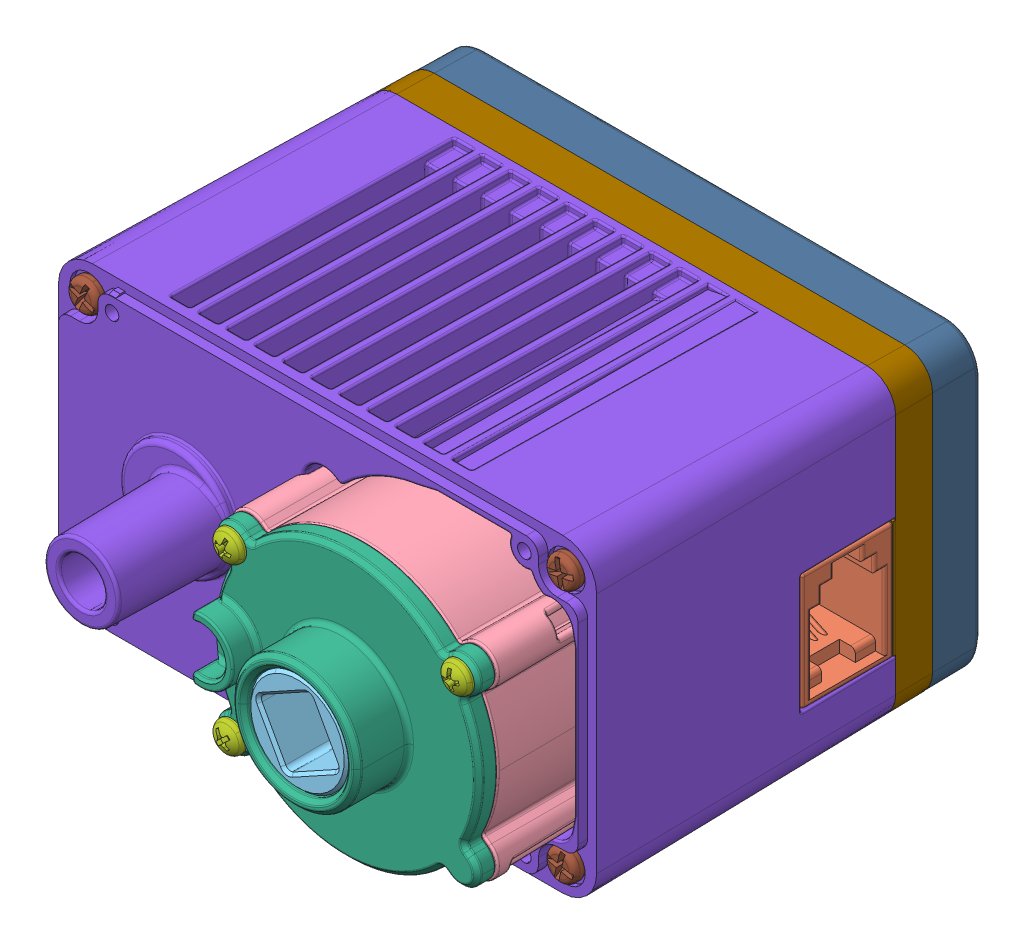
SolidWorks assembly V5 Smart Motor (276-4840) no cap 2, configuration Default. Lengths in mm.
Overall size (59.01 35.33 59.91).
19 component instances, 12 part files, 0 mates.
Components (placement in the parent):
- 276-4840-900 Rev6_Instruction.step-1: 276-4840-900 Rev6_Instruction.step [Default] at (-14.3 0 -17.2) size (52.79 15.94 38.15)
  - 276-4840-901 Rev6.step-1: 276-4840-901 Rev6.step [Default] at (10.75 -10.05 17.8) x (-1 0 0) z (0 0 1) size (49.9 1.6 38.15)
  - 276-4840-902 Rev2.step-1: 276-4840-902 Rev2.step [Default] at (31.25 -9.25 6.2) x (0 0 -1) z (0 -1 0) size (10.35 11.39 15.94)
  - 276-4840-022 Rev4.step-1: 276-4840-022 Rev4.step [Default] at (31.25 -9.25 6.2) x (0 0 -1) z (1 0 0) size (10.26 9.1 5.51)
- 276-4840-110 Rev10_Instruction.step-1: 276-4840-110 Rev10_Instruction.step [Default] at (12.7 0 14.7) size (35.33 35.33 31.1)
  - 276-4840-061 Rev7_Ring_Gear_Fixed01 .6 Rev3.step-1: 276-4840-061 Rev7_Ring_Gear_Fixed01 .6 Rev3.step [Default] at origin size (28.79 28.39 24.6)
  - 276-4840-018 Rev6.step-1: 276-4840-018 Rev6.step [Default] at (0 0 6.7) x (-0.483174 0.875524 0) z (0 0 1) size (26 26 12.3)
  - 276-4840-059 Rev2.step-1: 276-4840-059 Rev2.step [Default] at (0 0 10.3) size (28.4 28.4 8.5)
  - 276-4840-062 Rev1.step-1: 276-4840-062 Rev1.step [Default] at (-12.1353 8.8168 12.3) x (0.956835 -0.290632 0) z (-0.290632 -0.956835 0) size (3.2 6.56 3.2)
  - 276-4840-062 Rev1.step-2: 276-4840-062 Rev1.step [Default] at (12.1353 8.8168 12.3) x (0.978427 0.206591 0) z (0.206591 -0.978427 0) size (3.2 6.56 3.2)
  - 276-4840-062 Rev1.step-3: 276-4840-062 Rev1.step [Default] at (-12.1353 -8.8168 12.3) x (0.72563 0.688086 0) z (0.688086 -0.72563 0) size (3.2 6.56 3.2)
- 276-4840-001 Rev38.step-1: 276-4840-001 Rev38.step [Default] at origin size (57.3 33 46.9)
- 276-4840-005 Rev27.step-1: 276-4840-005 Rev27.step [Default] at (0 0 -17.95) size (56.17 31.87 12.9)
- 276-4840-004 Rev16.step-1: 276-4840-004 Rev16.step [Default] at (0 0 -19.2) size (56.01 31.71 9.21)
- 276-4840-009 Rev3.step-1: 276-4840-009 Rev3.step [Default] at (25.45 13.5 15.7) x (0.19987 -0.979823 0) z (-0.979823 -0.19987 0) size (3.4 41.31 4.34)
- 276-4840-009 Rev3.step-2: 276-4840-009 Rev3.step [Default] at (-25.45 -13.5 15.7) x (-0.998855 0.047836 0) z (0.047836 0.998855 0) size (3.4 41.31 4.34)
- 276-4840-009 Rev3.step-3: 276-4840-009 Rev3.step [Default] at (25.45 -13.5 15.7) x (-0.975374 0.220559 0) z (0.220559 0.975374 0) size (3.4 41.31 4.34)
- 276-4840-009 Rev3.step-4: 276-4840-009 Rev3.step [Default] at (-25.45 13.5 15.7) x (-0.922256 0.38658 0) z (0.38658 0.922256 0) size (3.4 41.31 4.34)
- 276-4840-025 Rev19.step-1: 276-4840-025 Rev19.step [Default] at (12.7 0 -22.63) x (-0.993315 0.115437 0) z (0 0 1) size (14.82 14.83 35.18)
